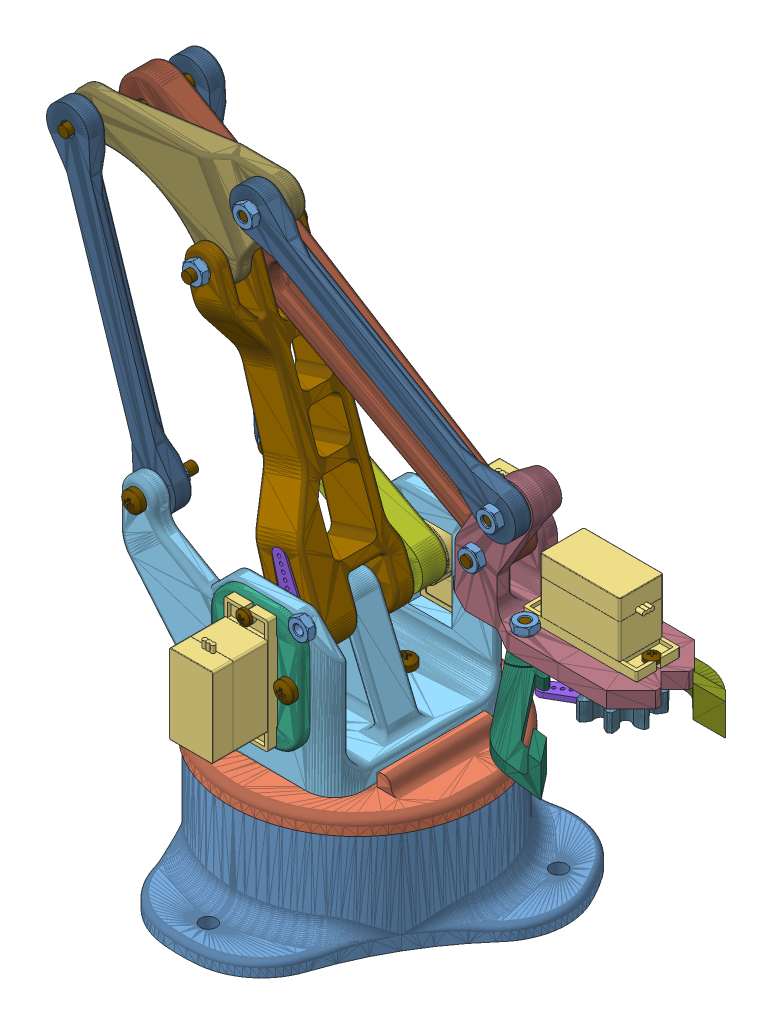
SolidWorks assembly Arm, configuration Default. Lengths in mm.
Overall size (174.72 168.21 117.68).
58 component instances, 19 part files, 132 mates.
Components (placement in the parent):
- EBA_01.00.010_basement-1: EBA_01.00.010_basement [Default] at (-51.5742 0 161.4746) x (1 0 0) z (0 1 0) size (94.67 87.46 31)
- EBA_01.00.011_round_plate-1: EBA_01.00.011_round_plate [Default] at (-40.2232 29.4 74.2148) x (0 0 1) z (0 1 0) size (72 72 8.5)
- microservoSG90-2: microservoSG90 [Default] at (-3.8619 1.6 115.6746) x (0 0 1) z (-1 0 0) size (32.3 29.8 12.5)
- microservoArmLong-1: microservoArmLong [A2] at (-3.8619 32.9 110.5746) x (0.999881 0 -0.01542) z (-0.01542 0 -0.999881) size (34.4 3.9 7)
- EBA_01.00.001-1: EBA_01.00.001 [Default] at (-45.8742 33.9 84.2868) x (0 0 1) z (0 1 0) size (52 61.1 52.63)
- microservoSG90-3: microservoSG90 [Default] at (-4.3132 59.1 63.8468) x (0 -1 0) z (-1 0 0) size (32.3 29.8 12.5)
- EBA_01.00.009_servo_plate-1: EBA_01.00.009_servo_plate [Default] at (-17.4932 41.73 84.5468) x (0 1 0) z (0 0 -1) size (34 26 2.5)
- microservoSG90-4: microservoSG90 [Default] at (-4.4132 59.1 157.2468) x (0 -1 0) z (1 0 0) size (32.3 29.8 12.5)
- EBA_01.00.009_servo_plate-2: EBA_01.00.009_servo_plate [Default] at (-17.4932 76.07 136.5468) x (0 -1 0) z (0 0 1) size (34 26 2.5)
- EBA_01.00.002_vertical_drive_arm-1: EBA_01.00.002_vertical_drive_arm [Default] at (-35.5624 90.0957 98.1843) x (0.863026 -0.505159 0) z (0 0 -1) size (46.49 12.99 7.5)
- microservoArm-1: microservoArm [A3] at (-4.3132 64.2 95.1468) x (-0.870713 0.491791 0) z (-0.491791 -0.870713 0) size (20.7 3.9 7)
- EBA_01.00.004_forward_drive_arm-1: EBA_01.00.004_forward_drive_arm [Default] at (5.2745 59.6273 130.0218) x (-0.337622 0.941282 0) z (-0.941282 -0.337622 0) size (92.46 29 15)
- microservoArm-2: microservoArm [A3] at (-4.4132 64.2 125.9468) x (-0.322675 0.94651 0) z (0.94651 0.322675 0) size (20.7 3.9 7)
- EBA_01.00.003_link-1: EBA_01.00.003_link [Default] at (-38.1599 73.4815 103.1718) x (-0.309528 0.95089 0) z (0 0 -1) size (92 12 5)
- EBA_01.00.003_link-2: EBA_01.00.003_link [Default] at (-44.1172 73.138 131.5718) x (-0.307997 0.951387 0) z (0 0 -1) size (92 12 5)
- EBA_01.00.005_horizontal_arm-1: EBA_01.00.005_horizontal_arm [Default] at (-69.6454 155.2282 107.8068) x (0.863665 -0.504067 0) z (0 0 1) size (127.5 15 8)
- EBA_01.00.006_triangular_link-1: EBA_01.00.006_triangular_link [Default] at (-71.5103 163.8915 125.2487) x (0 0 -1) z (-0.002811 -0.999996 0) size (9 58.25 29.23)
- EBA_01.00.003_link-3: EBA_01.00.003_link [Default] at (53.112 108.4946 125.8718) x (-0.863664 0.504069 0) z (0 0 -1) size (92 12 5)
- EBA_01.00.012_R01_claw_support-1: EBA_01.00.012_R01_claw_support [Default] at (33.9347 84.854 124.9718) x (0.999996 -0.002818 0) z (0.002818 0.999996 0) size (54 25 38.23)
- microservoSG90-5: microservoSG90 [Default] at (67.259 107.6102 112.3968) x (-0.999996 0.002818 0) z (0 0 1) size (32.3 29.8 12.5)
- EBA_01.00.015_drive_gear-1: EBA_01.00.015_drive_gear [Default] at (75.128 75.2329 98.3974) x (-0.834082 0.002351 0.551635) z (0.002818 0.999996 0) size (20 20 5)
- microservoArm-3: microservoArm [A3] at (72.2708 76.296 112.3968) x (-0.825477 0.002326 0.564431) z (-0.564429 0.001591 -0.82548) size (20.7 3.9 7)
- EBA_01.00.013_R01_right_finger-1: EBA_01.00.013_R01_right_finger [Default] at (92.0684 81.4952 152.2949) x (-0.616674 0.001738 -0.787216) z (0.002818 0.999996 0) size (58.42 14.02 9)
- EBA_01.00.014_R01_left_finger-1: EBA_01.00.014_R01_left_finger [Default] at (101.9721 81.7673 99.4596) x (-0.999986 0.002818 0.004425) z (0.002818 0.999996 0) size (58.42 14.5 9)
- EBA_01.00.016_R01_driven_gear-1: EBA_01.00.016_R01_driven_gear [Default] at (68.5811 76.8764 95.689) x (-0.999986 0.002818 0.004425) z (0.002818 0.999996 0) size (28 21.47 7)
- pan head cross recess screw_iso-1: pan head cross recess screw_iso [ISO 7045 - M3 x 10 - Z - 10N] at (54.479 79.2461 121.3968) x (0.002818 0.999996 0) z (-0.001886 0.000005 0.999998) size (12.35 5.6 5.6)
- pan head cross recess screw_iso-2: pan head cross recess screw_iso [ISO 7045 - M3 x 16 - Z - 16N] at (54.468 74.5461 103.2948) x (0.002818 0.999996 0) z (-0.001886 0.000005 0.999998) size (18.35 5.6 5.6)
- pan head cross recess screw_iso-5: pan head cross recess screw_iso [ISO 7045 - M2 x 8 - Z - 8N] at (81.4667 92.5701 112.3968) x (-0.002818 -0.999996 0) z (0.671239 -0.001892 -0.741238) size (9.57 4 4)
- pan head cross recess screw_iso-6: pan head cross recess screw_iso [ISO 7045 - M2 x 8 - Z - 8N] at (52.9668 92.6504 112.3968) x (-0.002818 -0.999996 0) z (-0.544965 0.001536 0.838457) size (9.57 4 4)
- pan head cross recess screw_iso-9: pan head cross recess screw_iso [ISO 7045 - M3 x 16 - Z - 16N] at (50.2419 117.1863 109.2468) x (0 0 1) z (0.914299 0.405039 0) size (18.35 5.6 5.6)
- pan head cross recess screw_iso-12: pan head cross recess screw_iso [ISO 7045 - M3 x 20 - Z - 20N] at (40.0374 99.9869 101.4468) x (0 0 1) z (0.914299 0.405039 0) size (22.35 5.6 5.6)
- pan head cross recess screw_iso-14: pan head cross recess screw_iso [ISO 7045 - M3 x 12 - Z - 12N] at (-18.8529 157.5111 113.4468) x (0 0 1) z (-0.914299 -0.405039 0) size (14.35 5.6 5.6)
- pan head cross recess screw_iso-15: pan head cross recess screw_iso [ISO 7045 - M3 x 12 - Z - 12N] at (-65.1062 157.6425 118.4468) x (0 0 1) z (0.914299 0.405039 0) size (14.35 5.6 5.6)
- pan head cross recess screw_iso-17: pan head cross recess screw_iso [ISO 7045 - M3 x 20 - Z - 20N] at (-59.2848 157.9522 95.7468) x (0 0 1) z (0.914299 0.405039 0) size (22.35 5.6 5.6)
- pan head cross recess screw_iso-20: pan head cross recess screw_iso [ISO 7045 - M3 x 16 - Z - 16N] at (-34.5209 81.8803 88.2468) x (0 0 1) z (0.917942 0.396714 0) size (18.35 5.6 5.6)
- pan head cross recess screw_iso-21: pan head cross recess screw_iso [ISO 7045 - M3 x 16 - Z - 16N] at (-40.4647 81.5309 138.9468) x (0 0 -1) z (1 0 0) size (18.35 5.6 5.6)
- pan head cross recess screw_iso-22: pan head cross recess screw_iso [ISO 7045 - M3 x 30 - Z - 25N] at (-29.0566 140.3098 101.4468) x (0 0 1) z (-0.380673 -0.92471 0) size (32.35 5.6 5.6)
- pan head cross recess screw_iso-26: pan head cross recess screw_iso [ISO 7045 - M3 x 8 - Z - 8N] at (5.1368 58.9 79.6468) x (0 0 1) z (0.914299 0.405039 0) size (10.35 5.6 5.6)
- pan head cross recess screw_iso-27: pan head cross recess screw_iso [ISO 7045 - M3 x 8 - Z - 8N] at (-13.8632 58.9 79.6468) x (0 0 1) z (-0.914299 -0.405039 0) size (10.35 5.6 5.6)
- pan head cross recess screw_iso-28: pan head cross recess screw_iso [ISO 7045 - M3 x 8 - Z - 8N] at (-13.8632 58.9 141.4468) x (0 0 -1) z (1 0 0) size (10.35 5.6 5.6)
- pan head cross recess screw_iso-29: pan head cross recess screw_iso [ISO 7045 - M3 x 8 - Z - 8N] at (5.1368 58.9 141.4468) x (0 0 -1) z (1 0 0) size (10.35 5.6 5.6)
- pan head cross recess screw_iso-31: pan head cross recess screw_iso [ISO 7045 - M3 x 8 - Z - 8N] at (-4.3632 41.3 96.5468) x (0 -1 0) z (0.546944 0 -0.837169) size (10.35 5.6 5.6)
- pan head cross recess screw_iso-32: pan head cross recess screw_iso [ISO 7045 - M3 x 8 - Z - 8N] at (-4.3642 41.3 124.5461) x (0 -1 0) z (0.546944 0 -0.837169) size (10.35 5.6 5.6)
- pan head cross recess screw_iso-33: pan head cross recess screw_iso [ISO 7045 - M2 x 8 - Z - 8N] at (-4.3132 73.35 77.8468) x (0 0 1) z (-0.914299 -0.405039 0) size (9.57 4 4)
- pan head cross recess screw_iso-34: pan head cross recess screw_iso [ISO 7045 - M2 x 8 - Z - 8N] at (-4.3132 44.85 77.8468) x (0 0 1) z (-0.914299 -0.405039 0) size (9.57 4 4)
- pan head cross recess screw_iso-35: pan head cross recess screw_iso [ISO 7045 - M2 x 8 - Z - 8N] at (-4.4132 73.35 143.2468) x (0 0 -1) z (0.902909 0.429831 0) size (9.57 4 4)
- pan head cross recess screw_iso-36: pan head cross recess screw_iso [ISO 7045 - M2 x 8 - Z - 8N] at (-4.4132 44.85 143.2468) x (0 0 -1) z (1 0 0) size (9.57 4 4)
- hex nut style 1 gradeab_iso-1: hex nut style 1 gradeab_iso [ISO - 4032 - M3 - W - N] at (50.2419 117.1863 181.5228) size (5.5 6.35 2.4)
- hex nut style 1 gradeab_iso-2: hex nut style 1 gradeab_iso [ISO - 4032 - M3 - W - N] at (54.5168 91.8461 103.2948) x (0.999994 -0.002818 -0.002211) z (0.002818 0.999996 0) size (5.5 6.35 2.4)
- hex nut style 1 gradeab_iso-4: hex nut style 1 gradeab_iso [ISO - 4032 - M3 - W - N] at (50.2419 117.1863 125.8468) x (0.919061 0.394115 0) z (0 0 -1) size (5.5 6.35 2.4)
- hex nut style 1 gradeab_iso-5: hex nut style 1 gradeab_iso [ISO - 4032 - M3 - W - N] at (54.5145 91.8461 121.3968) x (0.999994 -0.002818 -0.002211) z (0.002818 0.999996 0) size (5.5 6.35 2.4)
- hex nut style 1 gradeab_iso-6: hex nut style 1 gradeab_iso [ISO - 4032 - M3 - W - N] at (40.0374 99.9869 120.8468) x (0.919061 0.394115 0) z (0 0 -1) size (5.5 6.35 2.4)
- hex nut style 1 gradeab_iso-7: hex nut style 1 gradeab_iso [ISO - 4032 - M3 - W - N] at (-29.0566 140.3098 132.2468) x (1 0 0) z (0 0 1) size (5.5 6.35 2.4)
- hex nut style 1 gradeab_iso-8: hex nut style 1 gradeab_iso [ISO - 4032 - M3 - W - N] at (-18.8529 157.5111 128.2468) x (1 0 0) z (0 0 1) size (5.5 6.35 2.4)
- hex nut style 1 gradeab_iso-9: hex nut style 1 gradeab_iso [ISO - 4032 - M3 - W - N] at (-40.4647 81.5309 126.5468) size (5.5 6.35 2.4)
- hex nut style 1 gradeab_iso-10: hex nut style 1 gradeab_iso [ISO - 4032 - M3 - W - N] at (-34.5209 81.8803 105.5468) size (5.5 6.35 2.4)
- hex nut style 1 gradeab_iso-11: hex nut style 1 gradeab_iso [ISO - 4032 - M3 - W - N] at (-13.8632 58.9 130.6468) x (1 0 0) z (0 0 -1) size (5.5 6.35 2.4)
- hex nut style 1 gradeab_iso-12: hex nut style 1 gradeab_iso [ISO - 4032 - M3 - W - N] at (5.1368 58.9 130.6468) x (0.5 0.866025 0) z (0 0 -1) size (5.5 6.35 2.4)
Mates (geometry in assembly coordinates):
- Coincidente13: coincident anti-aligned: plane of EBA_01.00.010_basement-1 through (-51.5742 18.2 161.4746) normal (0 1 0); plane of microservoSG90-2 through (-3.8619 18.2 101.4246) normal (0 -1 0)
- Coincidente14: coincident anti-aligned: plane of microservoSG90-2 through (-3.8619 31.4 110.5746) normal (0 1 0); plane of microservoArmLong-1 through (-3.8619 31.4 110.5746) normal (0 -1 0)
- Coincidente15: coincident anti-aligned: plane of EBA_01.00.011_round_plate-1 through (-40.2232 32.9 74.2148) normal (0 -1 0); plane of microservoArmLong-1 through (-19.0601 32.9 110.809) normal (0 1 0)
- Coincidente18: coincident anti-aligned: plane of EBA_01.00.010_basement-1 through (-10.0619 0 161.4746) normal (1 0 0); plane of microservoSG90-2 through (-10.0619 17.2 104.3746) normal (-1 0 0)
- Coincidente19: coincident anti-aligned: plane of EBA_01.00.010_basement-1 through (-51.5742 0 104.3746) normal (0 0 1); plane of microservoSG90-2 through (-10.0619 17.2 104.3746) normal (0 0 -1)
- Coincidente20: coincident aligned: circle of microservoSG90-2; cylinder of microservoArmLong-1 through (-3.8619 29 110.5746) axis (0 1 0) radius 2.45
- Concentrico9: concentric aligned: circle of EBA_01.00.011_round_plate-1; circle of microservoArmLong-1
- Parallelo1: parallel anti-aligned: plane of EBA_01.00.011_round_plate-1 through (-36.5083 29.4 116.6765) normal (-0.087156 0 -0.996195); plane of microservoArmLong-1 through (-1.9479 29 113.5049) normal (0.087156 0 0.996195)
- Coincidente22: coincident anti-aligned: plane of EBA_01.00.011_round_plate-1 through (-40.2232 33.9 74.2148) normal (0 1 0); plane of EBA_01.00.001-1 through (-45.8742 33.9 84.2868) normal (0 -1 0)
- Coincidente23: coincident anti-aligned: plane of EBA_01.00.011_round_plate-1 through (-24.3632 29.4 74.2148) normal (1 0 0); plane of EBA_01.00.001-1 through (-24.3632 33.9 84.2868) normal (-1 0 0)
- Blocca1: lock: unknown of EBA_01.00.011_round_plate-1; unknown of EBA_01.00.001-1
- Coincidente28: coincident anti-aligned: plane of EBA_01.00.010_basement-1 through (-51.5742 0 161.4746) normal (0 -1 0); plane of assembly through (0 0 0) normal (0 1 0)
- Coincidente29: coincident anti-aligned: plane of EBA_01.00.001-1 through (-45.8742 33.9 84.5468) normal (0 0 -1); plane of EBA_01.00.009_servo_plate-1 through (-17.4932 41.73 84.5468) normal (0 0 1)
- Coincidente30: coincident: line of EBA_01.00.001-1 through (1.8868 47.4 84.5468) axis (0 1 0); plane of EBA_01.00.009_servo_plate-1 through (1.8868 41.73 84.5468) normal (-1 0 0)
- Coincidente31: coincident aligned: plane of EBA_01.00.001-1 through (-45.8742 47.4 84.2868) normal (0 1 0); plane of EBA_01.00.009_servo_plate-1 through (-17.4932 47.4 84.5468) normal (0 1 0)
- Coincidente33: coincident anti-aligned: plane of EBA_01.00.001-1 through (-45.8742 70.4 84.2868) normal (0 -1 0); plane of microservoSG90-3 through (1.8868 70.4 86.1468) normal (0 1 0)
- Coincidente34: coincident anti-aligned: plane of EBA_01.00.001-1 through (1.8868 33.9 84.2868) normal (-1 0 0); plane of microservoSG90-3 through (1.8868 70.4 79.4468) normal (1 0 0)
- Coincidente36: coincident anti-aligned: plane of EBA_01.00.001-1 through (-45.8742 33.9 136.5468) normal (0 0 1); plane of EBA_01.00.009_servo_plate-2 through (-17.4932 76.07 136.5468) normal (0 0 -1)
- Coincidente37: coincident aligned: plane of EBA_01.00.001-1 through (-45.8742 70.4 84.2868) normal (0 -1 0); plane of EBA_01.00.009_servo_plate-2 through (-17.4932 70.4 136.5468) normal (0 -1 0)
- Coincidente38: coincident aligned: plane of EBA_01.00.001-1 through (1.8868 33.9 84.2868) normal (-1 0 0); plane of EBA_01.00.009_servo_plate-2 through (1.8868 76.07 136.5468) normal (-1 0 0)
- Coincidente42: coincident anti-aligned: plane of microservoSG90-3 through (-4.3132 59.1 82.0468) normal (0 0 1); plane of EBA_01.00.009_servo_plate-1 through (-17.4932 41.73 82.0468) normal (0 0 -1)
- Coincidente43: coincident anti-aligned: plane of EBA_01.00.001-1 through (-10.6132 33.9 84.2868) normal (1 0 0); plane of microservoSG90-4 through (-10.6132 70.4 141.6468) normal (-1 0 0)
- Coincidente44: coincident anti-aligned: plane of microservoSG90-4 through (-4.4132 59.1 139.0468) normal (0 0 -1); plane of EBA_01.00.009_servo_plate-2 through (-17.4932 76.07 139.0468) normal (0 0 1)
- Coincidente45: coincident anti-aligned: plane of EBA_01.00.001-1 through (-45.8742 70.4 84.2868) normal (0 -1 0); plane of microservoSG90-4 through (1.7868 70.4 141.6468) normal (0 1 0)
- Concentrico10: concentric anti-aligned: cylinder of microservoSG90-3 through (-4.3132 64.2 93.6468) axis (0 0 -1) radius 2.45; cylinder of microservoArm-1 through (-4.3132 64.2 91.2468) axis (0 0 1) radius 2.45
- Coincidente46: coincident anti-aligned: plane of microservoSG90-3 through (-4.3132 64.2 93.6468) normal (0 0 1); plane of microservoArm-1 through (-4.3132 64.2 93.6468) normal (0 0 -1)
- Concentrico11: concentric anti-aligned: circle of EBA_01.00.002_vertical_drive_arm-1; circle of microservoArm-1
- Coincidente47: coincident anti-aligned: plane of EBA_01.00.002_vertical_drive_arm-1 through (-35.5624 90.0957 95.1468) normal (0 0 -1); plane of microservoArm-1 through (8.9216 56.7248 95.1468) normal (0 0 1)
- Parallelo2: parallel anti-aligned: plane of EBA_01.00.002_vertical_drive_arm-1 through (-38.4159 84.0704 98.1843) normal (-0.428019 -0.90377 0); plane of microservoArm-1 through (-4.4848 67.6958 91.2468) normal (0.428019 0.90377 0)
- Concentrico12: concentric anti-aligned: cylinder of microservoSG90-4 through (-4.4132 64.2 127.4468) axis (0 0 1) radius 2.45; cylinder of microservoArm-2 through (-4.4132 64.2 129.8468) axis (0 0 -1) radius 2.45
- Coincidente49: coincident anti-aligned: plane of microservoSG90-4 through (-4.4132 64.2 127.4468) normal (0 0 -1); plane of microservoArm-2 through (-4.4132 64.2 127.4468) normal (0 0 1)
- Concentrico13: concentric anti-aligned: circle of EBA_01.00.004_forward_drive_arm-1; cylinder of microservoArm-2 through (-4.4132 64.2 129.8468) axis (0 0 -1) radius 3.5
- Parallelo3: parallel anti-aligned: plane of EBA_01.00.004_forward_drive_arm-1 through (1.7978 58.1557 130.0218) normal (-0.920905 -0.389787 0); plane of microservoArm-2 through (-7.4249 79.2323 129.8468) normal (0.920905 0.389787 0)
- Coincidente53: coincident aligned: plane of EBA_01.00.004_forward_drive_arm-1 through (5.2745 59.6273 127.3468) normal (0 0 1); plane of microservoArm-2 through (0.4915 49.8131 127.3468) normal (0 0 1)
- Concentrico14: concentric aligned: circle of EBA_01.00.002_vertical_drive_arm-1; circle of EBA_01.00.003_link-1
- Coincidente54: coincident anti-aligned: plane of EBA_01.00.002_vertical_drive_arm-1 through (-35.5624 90.0957 98.1468) normal (0 0 1); plane of EBA_01.00.003_link-1 through (-38.1599 73.4815 98.1468) normal (0 0 -1)
- Coincidente55: coincident anti-aligned: plane of EBA_01.00.001-1 through (-45.8742 33.9 131.5468) normal (0 0 -1); plane of EBA_01.00.003_link-2 through (-44.1172 73.138 131.5468) normal (0 0 1)
- Concentrico15: concentric anti-aligned: circle of EBA_01.00.001-1; circle of EBA_01.00.003_link-2
- Concentrico18: concentric aligned: circle of EBA_01.00.004_forward_drive_arm-1; circle of EBA_01.00.005_horizontal_arm-1
- Coincidente60: coincident anti-aligned: plane of EBA_01.00.004_forward_drive_arm-1 through (5.2745 59.6273 107.8468) normal (0 0 1); plane of EBA_01.00.005_horizontal_arm-1 through (-69.6454 155.2282 107.8468) normal (0 0 -1)
- Concentrico19: concentric anti-aligned: circle of EBA_01.00.003_link-1; circle of EBA_01.00.005_horizontal_arm-1
- Concentrico20: concentric anti-aligned: circle of EBA_01.00.004_forward_drive_arm-1; circle of EBA_01.00.006_triangular_link-1
- Coincidente61: coincident anti-aligned: plane of EBA_01.00.004_forward_drive_arm-1 through (5.2745 59.6273 120.8468) normal (0 0 1); plane of EBA_01.00.006_triangular_link-1 through (-71.5103 163.8915 120.8468) normal (0 0 -1)
- Concentrico21: concentric aligned: circle of EBA_01.00.003_link-2; circle of EBA_01.00.006_triangular_link-1
- Concentrico22: concentric aligned: circle of EBA_01.00.006_triangular_link-1; circle of EBA_01.00.003_link-3
- Coincidente62: coincident anti-aligned: plane of EBA_01.00.006_triangular_link-1 through (-71.5103 163.8915 120.8468) normal (0 0 1); plane of EBA_01.00.003_link-3 through (53.112 108.4946 120.8468) normal (0 0 -1)
- Concentrico23: concentric anti-aligned: circle of EBA_01.00.003_link-3; circle of EBA_01.00.012_R01_claw_support-1
- Coincidente63: coincident anti-aligned: plane of EBA_01.00.003_link-3 through (53.112 108.4946 120.8468) normal (0 0 -1); plane of EBA_01.00.012_R01_claw_support-1 through (33.9347 84.854 120.8468) normal (0 0 1)
- Concentrico24: concentric aligned: circle of EBA_01.00.005_horizontal_arm-1; circle of EBA_01.00.012_R01_claw_support-1
- Coincidente65: coincident anti-aligned: plane of EBA_01.00.012_R01_claw_support-1 through (78.4945 84.7285 124.9718) normal (-0.999996 0.002818 0); plane of microservoSG90-5 through (78.515 91.9784 118.5968) normal (0.999996 -0.002818 0)
- Coincidente66: coincident anti-aligned: plane of EBA_01.00.012_R01_claw_support-1 through (33.9347 84.854 118.5968) normal (0 0 -1); plane of microservoSG90-5 through (78.515 91.9784 118.5968) normal (0 0 1)
- Concentrico25: concentric anti-aligned: cylinder of microservoSG90-5 through (72.275 77.796 112.3968) axis (0.002818 0.999996 0) radius 2.45; cylinder of microservoArm-3 through (72.2817 80.196 112.3968) axis (-0.002818 -0.999996 0) radius 2.45
- Coincidente67: coincident anti-aligned: plane of microservoSG90-5 through (72.275 77.796 112.3968) normal (-0.002818 -0.999996 0); plane of microservoArm-3 through (72.275 77.796 112.3968) normal (0.002818 0.999996 0)
- Concentrico26: concentric anti-aligned: circle of EBA_01.00.015_drive_gear-1; cylinder of microservoArm-3 through (72.2817 80.196 112.3968) axis (-0.002818 -0.999996 0) radius 3.5
- Coincidente68: coincident anti-aligned: plane of EBA_01.00.015_drive_gear-1 through (75.131 76.2879 98.3974) normal (0.002818 0.999996 0); plane of microservoArm-3 through (84.818 76.2606 103.8175) normal (-0.002818 -0.999996 0)
- Parallelo4: parallel anti-aligned: plane of EBA_01.00.015_drive_gear-1 through (78.8291 75.2224 103.0537) normal (0.622229 -0.001754 0.782834); plane of microservoArm-3 through (58.6056 80.2345 119.3252) normal (-0.622229 0.001754 -0.782834)
- Concentrico27: concentric anti-aligned: circle of EBA_01.00.012_R01_claw_support-1; circle of EBA_01.00.013_R01_right_finger-1
- Coincidente74: coincident anti-aligned: plane of EBA_01.00.012_R01_claw_support-1 through (33.9351 85.004 124.9718) normal (-0.002818 -0.999996 0); plane of EBA_01.00.013_R01_right_finger-1 through (92.0779 84.8402 152.2949) normal (0.002818 0.999996 0)
- Concentrico28: concentric anti-aligned: circle of EBA_01.00.012_R01_claw_support-1; circle of EBA_01.00.014_R01_left_finger-1
- Coincidente75: coincident anti-aligned: plane of EBA_01.00.012_R01_claw_support-1 through (33.9351 85.004 124.9718) normal (-0.002818 -0.999996 0); plane of EBA_01.00.014_R01_left_finger-1 through (101.9806 84.8123 99.4596) normal (0.002818 0.999996 0)
- Coincidente76: coincident anti-aligned: plane of EBA_01.00.012_R01_claw_support-1 through (33.9478 89.504 124.9718) normal (0.002818 0.999996 0); plane of microservoSG90-5 through (67.2077 89.4103 112.3968) normal (-0.002818 -0.999996 0)
- Concentrico29: concentric anti-aligned: circle of EBA_01.00.012_R01_claw_support-1; circle of EBA_01.00.016_R01_driven_gear-1
- Parallelo5: parallel anti-aligned: plane of EBA_01.00.014_R01_left_finger-1 through (101.9726 81.7673 99.5846) normal (-0.004425 0.000012 -0.99999); plane of EBA_01.00.016_R01_driven_gear-1 through (68.5986 76.8763 99.6322) normal (0.004425 -0.000012 0.99999)
- Coincidente78: coincident anti-aligned: plane of EBA_01.00.014_R01_left_finger-1 through (101.9722 81.8123 99.4596) normal (-0.002818 -0.999996 0); plane of EBA_01.00.016_R01_driven_gear-1 through (68.5953 81.9064 95.689) normal (0.002818 0.999996 0)
- Concentrico31: concentric aligned: circle of EBA_01.00.012_R01_claw_support-1; circle of pan head cross recess screw_iso-1
- Coincidente81: coincident anti-aligned: plane of EBA_01.00.013_R01_right_finger-1 through (92.0686 81.5402 152.2949) normal (-0.002818 -0.999996 0); plane of pan head cross recess screw_iso-1 through (52.9858 81.6503 121.394) normal (0.002818 0.999996 0)
- Concentrico32: concentric aligned: circle of EBA_01.00.012_R01_claw_support-1; cylinder of pan head cross recess screw_iso-2 through (54.3964 49.1462 103.2948) axis (-0.002818 -0.999996 0) radius 1.5
- Coincidente82: coincident anti-aligned: plane of EBA_01.00.016_R01_driven_gear-1 through (68.5812 76.9064 95.689) normal (-0.002818 -0.999996 0); plane of pan head cross recess screw_iso-2 through (52.9748 76.9504 103.2919) normal (0.002818 0.999996 0)
- Concentrico34: concentric anti-aligned: cylinder of microservoSG90-5 through (81.4749 95.4929 112.3968) axis (-0.002818 -0.999996 0) radius 1; cylinder of pan head cross recess screw_iso-5 through (81.5382 117.97 112.3968) axis (0.002818 0.999996 0) radius 1
- Coincidente85: coincident anti-aligned: plane of microservoSG90-5 through (81.4621 90.9701 112.3968) normal (0.002818 0.999996 0); plane of pan head cross recess screw_iso-5 through (80.7209 90.9722 111.7256) normal (-0.002818 -0.999996 0)
- Concentrico35: concentric anti-aligned: cylinder of microservoSG90-5 through (52.975 95.5732 112.3968) axis (-0.002818 -0.999996 0) radius 1; cylinder of pan head cross recess screw_iso-6 through (53.0383 118.0503 112.3968) axis (0.002818 0.999996 0) radius 1
- Coincidente86: coincident anti-aligned: plane of microservoSG90-5 through (52.9623 91.0505 112.3968) normal (0.002818 0.999996 0); plane of pan head cross recess screw_iso-6 through (53.8007 91.0481 112.9418) normal (-0.002818 -0.999996 0)
- Concentrico38: concentric aligned: circle of EBA_01.00.003_link-3; cylinder of pan head cross recess screw_iso-9 through (50.2419 117.1863 83.8468) axis (0 0 -1) radius 1.5
- Coincidente88: coincident anti-aligned: plane of EBA_01.00.012_R01_claw_support-1 through (33.9347 84.854 111.6468) normal (0 0 -1); plane of pan head cross recess screw_iso-9 through (50.8495 115.8149 111.6468) normal (0 0 1)
- Concentrico41: concentric anti-aligned: circle of EBA_01.00.005_horizontal_arm-1; cylinder of pan head cross recess screw_iso-12 through (40.0374 99.9869 76.0468) axis (0 0 -1) radius 1.5
- Coincidente93: coincident anti-aligned: plane of EBA_01.00.012_R01_claw_support-1 through (33.9347 84.854 103.8468) normal (0 0 -1); plane of pan head cross recess screw_iso-12 through (40.6449 98.6155 103.8468) normal (0 0 1)
- Concentrico43: concentric aligned: circle of EBA_01.00.003_link-3; cylinder of pan head cross recess screw_iso-14 through (-18.8529 157.5111 88.0468) axis (0 0 -1) radius 1.5
- Coincidente95: coincident anti-aligned: plane of EBA_01.00.006_triangular_link-1 through (-71.5103 163.8915 115.8468) normal (0 0 -1); plane of pan head cross recess screw_iso-14 through (-19.4604 158.8826 115.8468) normal (0 0 1)
- Concentrico44: concentric aligned: circle of EBA_01.00.003_link-2; cylinder of pan head cross recess screw_iso-15 through (-65.1062 157.6425 93.0468) axis (0 0 -1) radius 1.5
- Coincidente96: coincident anti-aligned: plane of EBA_01.00.006_triangular_link-1 through (-71.5103 163.8915 120.8468) normal (0 0 -1); plane of pan head cross recess screw_iso-15 through (-64.4986 156.2711 120.8468) normal (0 0 1)
- Concentrico47: concentric anti-aligned: circle of EBA_01.00.005_horizontal_arm-1; cylinder of pan head cross recess screw_iso-17 through (-59.2848 157.9522 70.3468) axis (0 0 -1) radius 1.5
- Coincidente98: coincident anti-aligned: plane of EBA_01.00.003_link-1 through (-38.1599 73.4815 98.1468) normal (0 0 -1); plane of pan head cross recess screw_iso-17 through (-58.6773 156.5807 98.1468) normal (0 0 1)
- Concentrico49: concentric aligned: circle of EBA_01.00.003_link-1; cylinder of pan head cross recess screw_iso-20 through (-34.5209 81.8803 62.8468) axis (0 0 -1) radius 1.5
- Coincidente100: coincident anti-aligned: plane of EBA_01.00.002_vertical_drive_arm-1 through (-35.5624 90.0957 90.6468) normal (0 0 -1); plane of pan head cross recess screw_iso-20 through (-33.9258 80.5034 90.6468) normal (0 0 1)
- Concentrico50: concentric aligned: circle of EBA_01.00.001-1; cylinder of pan head cross recess screw_iso-21 through (-40.4647 81.5309 164.3468) axis (0 0 1) radius 1.5
- Coincidente101: coincident anti-aligned: plane of EBA_01.00.001-1 through (-45.8742 33.9 136.5468) normal (0 0 1); plane of pan head cross recess screw_iso-21 through (-40.4647 83.0309 136.5468) normal (0 0 -1)
- Concentrico51: concentric aligned: circle of EBA_01.00.006_triangular_link-1; cylinder of pan head cross recess screw_iso-22 through (-29.0566 140.3098 76.0468) axis (0 0 -1) radius 1.5
- Coincidente102: coincident anti-aligned: plane of EBA_01.00.004_forward_drive_arm-1 through (5.2745 59.6273 103.8468) normal (0 0 -1); plane of pan head cross recess screw_iso-22 through (-30.4436 140.8808 103.8468) normal (0 0 1)
- Coincidente105: coincident anti-aligned: plane of EBA_01.00.009_servo_plate-1 through (-17.4932 41.73 82.0468) normal (0 0 -1); plane of pan head cross recess screw_iso-26 through (5.7443 57.5286 82.0468) normal (0 0 1)
- Concentrico54: concentric aligned: circle of EBA_01.00.009_servo_plate-1; cylinder of pan head cross recess screw_iso-26 through (5.1368 58.9 54.2468) axis (0 0 -1) radius 1.5
- Coincidente107: coincident anti-aligned: plane of EBA_01.00.009_servo_plate-1 through (-17.4932 41.73 82.0468) normal (0 0 -1); plane of pan head cross recess screw_iso-27 through (-14.4708 60.2714 82.0468) normal (0 0 1)
- Concentrico55: concentric aligned: circle of EBA_01.00.009_servo_plate-1; cylinder of pan head cross recess screw_iso-27 through (-13.8632 58.9 54.2468) axis (0 0 -1) radius 1.5
- Concentrico56: concentric aligned: circle of EBA_01.00.009_servo_plate-2; cylinder of pan head cross recess screw_iso-28 through (-13.8632 58.9 166.8468) axis (0 0 1) radius 1.5
- Coincidente108: coincident anti-aligned: plane of EBA_01.00.009_servo_plate-2 through (-17.4932 76.07 139.0468) normal (0 0 1); plane of pan head cross recess screw_iso-28 through (-13.8632 60.4 139.0468) normal (0 0 -1)
- Concentrico57: concentric aligned: circle of EBA_01.00.009_servo_plate-2; cylinder of pan head cross recess screw_iso-29 through (5.1368 58.9 166.8468) axis (0 0 1) radius 1.5
- Coincidente109: coincident anti-aligned: plane of EBA_01.00.009_servo_plate-2 through (-17.4932 76.07 139.0468) normal (0 0 1); plane of pan head cross recess screw_iso-29 through (5.1368 60.4 139.0468) normal (0 0 -1)
- Concentrico58: concentric aligned: circle of EBA_01.00.001-1; cylinder of pan head cross recess screw_iso-31 through (-4.3632 66.7 96.5468) axis (0 1 0) radius 1.5
- Coincidente110: coincident anti-aligned: plane of EBA_01.00.001-1 through (-45.8742 38.9 84.2868) normal (0 1 0); plane of pan head cross recess screw_iso-31 through (-5.619 38.9 95.7264) normal (0 -1 0)
- Concentrico60: concentric aligned: circle of EBA_01.00.001-1; cylinder of pan head cross recess screw_iso-32 through (-4.3642 66.7 124.5461) axis (0 1 0) radius 1.5
- Coincidente111: coincident anti-aligned: plane of EBA_01.00.001-1 through (-45.8742 38.9 84.2868) normal (0 1 0); plane of pan head cross recess screw_iso-32 through (-5.62 38.9 123.7257) normal (0 -1 0)
- Coincidente112: coincident anti-aligned: plane of microservoSG90-3 through (-4.3132 59.1 79.4468) normal (0 0 -1); plane of pan head cross recess screw_iso-33 through (-4.7183 74.2643 79.4468) normal (0 0 1)
- Concentrico62: concentric anti-aligned: cylinder of microservoSG90-3 through (-4.3132 73.35 75.9241) axis (0 0 1) radius 1; cylinder of pan head cross recess screw_iso-33 through (-4.3132 73.35 52.4468) axis (0 0 -1) radius 1
- Coincidente113: coincident anti-aligned: plane of microservoSG90-3 through (-4.3132 59.1 79.4468) normal (0 0 -1); plane of pan head cross recess screw_iso-34 through (-4.7183 45.7643 79.4468) normal (0 0 1)
- Concentrico63: concentric anti-aligned: cylinder of microservoSG90-3 through (-4.3132 44.85 75.9241) axis (0 0 1) radius 1; cylinder of pan head cross recess screw_iso-34 through (-4.3132 44.85 52.4468) axis (0 0 -1) radius 1
- Concentrico64: concentric anti-aligned: cylinder of microservoSG90-4 through (-4.4132 73.35 145.1696) axis (0 0 -1) radius 1; cylinder of pan head cross recess screw_iso-35 through (-4.4132 73.35 168.6468) axis (0 0 1) radius 1
- Coincidente114: coincident anti-aligned: plane of microservoSG90-4 through (-4.4132 59.1 141.6468) normal (0 0 1); plane of pan head cross recess screw_iso-35 through (-4.843 74.2529 141.6468) normal (0 0 -1)
- Coincidente115: coincident anti-aligned: plane of microservoSG90-4 through (-4.4132 59.1 141.6468) normal (0 0 1); plane of pan head cross recess screw_iso-36 through (-4.4132 45.85 141.6468) normal (0 0 -1)
- Concentrico65: concentric anti-aligned: cylinder of microservoSG90-4 through (-4.4132 44.85 145.1696) axis (0 0 -1) radius 1; cylinder of pan head cross recess screw_iso-36 through (-4.4132 44.85 168.6468) axis (0 0 1) radius 1
- Concentrico66: concentric anti-aligned: cylinder of pan head cross recess screw_iso-2 through (54.3964 49.1462 103.2948) axis (-0.002818 -0.999996 0) radius 1.5; cylinder of hex nut style 1 gradeab_iso-2 through (54.51 89.4461 103.2948) axis (0.002818 0.999996 0) radius 1.25
- Coincidente116: coincident anti-aligned: plane of EBA_01.00.012_R01_claw_support-1 through (33.9478 89.504 124.9718) normal (0.002818 0.999996 0); plane of hex nut style 1 gradeab_iso-2 through (54.503 89.4461 100.1193) normal (-0.002818 -0.999996 0)
- Concentrico68: concentric anti-aligned: cylinder of pan head cross recess screw_iso-9 through (50.2419 117.1863 83.8468) axis (0 0 -1) radius 1.5; cylinder of hex nut style 1 gradeab_iso-1 through (50.2419 117.1863 179.1228) axis (0 0 1) radius 1.25
- Concentrico69: concentric aligned: cylinder of pan head cross recess screw_iso-9 through (50.2419 117.1863 83.8468) axis (0 0 -1) radius 1.5; cylinder of hex nut style 1 gradeab_iso-4 through (50.2419 117.1863 128.2468) axis (0 0 -1) radius 1.25
- Coincidente118: coincident anti-aligned: plane of EBA_01.00.003_link-3 through (53.112 108.4946 125.8468) normal (0 0 1); plane of hex nut style 1 gradeab_iso-4 through (51.4934 114.2679 125.8468) normal (0 0 -1)
- Concentrico70: concentric anti-aligned: cylinder of pan head cross recess screw_iso-1 through (54.4074 53.8462 121.3968) axis (-0.002818 -0.999996 0) radius 1.5; cylinder of hex nut style 1 gradeab_iso-5 through (54.5077 89.4461 121.3968) axis (0.002818 0.999996 0) radius 1.25
- Coincidente119: coincident anti-aligned: plane of EBA_01.00.012_R01_claw_support-1 through (33.9478 89.504 124.9718) normal (0.002818 0.999996 0); plane of hex nut style 1 gradeab_iso-5 through (54.5007 89.4461 118.2214) normal (-0.002818 -0.999996 0)
- Concentrico71: concentric anti-aligned: circle of EBA_01.00.012_R01_claw_support-1; cylinder of hex nut style 1 gradeab_iso-6 through (40.0374 99.9869 123.2468) axis (0 0 -1) radius 1.25
- Coincidente120: coincident anti-aligned: plane of EBA_01.00.012_R01_claw_support-1 through (33.9347 84.854 120.8468) normal (0 0 1); plane of hex nut style 1 gradeab_iso-6 through (41.2889 97.0685 120.8468) normal (0 0 -1)
- Concentrico72: concentric anti-aligned: cylinder of pan head cross recess screw_iso-14 through (-18.8529 157.5111 88.0468) axis (0 0 -1) radius 1.5; cylinder of hex nut style 1 gradeab_iso-8 through (-18.8529 157.5111 125.8468) axis (0 0 1) radius 1.25
- Coincidente121: coincident anti-aligned: plane of EBA_01.00.003_link-3 through (53.112 108.4946 125.8468) normal (0 0 1); plane of hex nut style 1 gradeab_iso-8 through (-18.8529 160.6866 125.8468) normal (0 0 -1)
- Concentrico73: concentric anti-aligned: cylinder of pan head cross recess screw_iso-22 through (-29.0566 140.3098 76.0468) axis (0 0 -1) radius 1.5; cylinder of hex nut style 1 gradeab_iso-7 through (-29.0566 140.3098 129.8468) axis (0 0 1) radius 1.25
- Coincidente122: coincident anti-aligned: plane of EBA_01.00.004_forward_drive_arm-1 through (5.2745 59.6273 129.8468) normal (0 0 1); plane of hex nut style 1 gradeab_iso-7 through (-29.0566 143.4852 129.8468) normal (0 0 -1)
- Concentrico74: concentric aligned: cylinder of pan head cross recess screw_iso-21 through (-40.4647 81.5309 164.3468) axis (0 0 1) radius 1.5; circle of hex nut style 1 gradeab_iso-9
- Coincidente123: coincident anti-aligned: plane of EBA_01.00.003_link-2 through (-44.1172 73.138 126.5468) normal (0 0 -1); plane of hex nut style 1 gradeab_iso-9 through (-40.4647 84.7064 126.5468) normal (0 0 1)
- Concentrico75: concentric anti-aligned: cylinder of pan head cross recess screw_iso-20 through (-34.5209 81.8803 62.8468) axis (0 0 -1) radius 1.5; cylinder of hex nut style 1 gradeab_iso-10 through (-34.5209 81.8803 103.1468) axis (0 0 1) radius 1.25
- Coincidente124: coincident anti-aligned: plane of EBA_01.00.003_link-1 through (-38.1599 73.4815 103.1468) normal (0 0 1); plane of hex nut style 1 gradeab_iso-10 through (-34.5209 85.0557 103.1468) normal (0 0 -1)
- Concentrico76: concentric anti-aligned: cylinder of pan head cross recess screw_iso-29 through (5.1368 58.9 166.8468) axis (0 0 1) radius 1.5; circle of hex nut style 1 gradeab_iso-12
- Coincidente125: coincident anti-aligned: plane of EBA_01.00.001-1 through (-45.8742 33.9 133.0468) normal (0 0 -1); plane of hex nut style 1 gradeab_iso-12 through (7.8868 57.3123 133.0468) normal (0 0 1)
- Concentrico77: concentric anti-aligned: cylinder of pan head cross recess screw_iso-28 through (-13.8632 58.9 166.8468) axis (0 0 1) radius 1.5; circle of hex nut style 1 gradeab_iso-11
- Coincidente126: coincident anti-aligned: plane of EBA_01.00.001-1 through (-45.8742 33.9 133.0468) normal (0 0 -1); plane of hex nut style 1 gradeab_iso-11 through (-13.8632 55.7246 133.0468) normal (0 0 1)
- Parallelo8: parallel anti-aligned: plane of EBA_01.00.001-1 through (-50.1218 41.257 84.2868) normal (0.5 -0.866025 0); plane of hex nut style 1 gradeab_iso-11 through (-16.6132 60.4877 133.0468) normal (-0.5 0.866025 0)
- Parallelo9: parallel anti-aligned: plane of EBA_01.00.001-1 through (-45.3718 33.0298 84.2868) normal (0.5 -0.866025 0); plane of hex nut style 1 gradeab_iso-12 through (2.3868 60.4877 133.0468) normal (-0.5 0.866025 0)
- Parallel1: parallel anti-aligned: plane of EBA_01.00.004_forward_drive_arm-1 through (5.2745 59.6273 103.8468) normal (0 0 -1)
